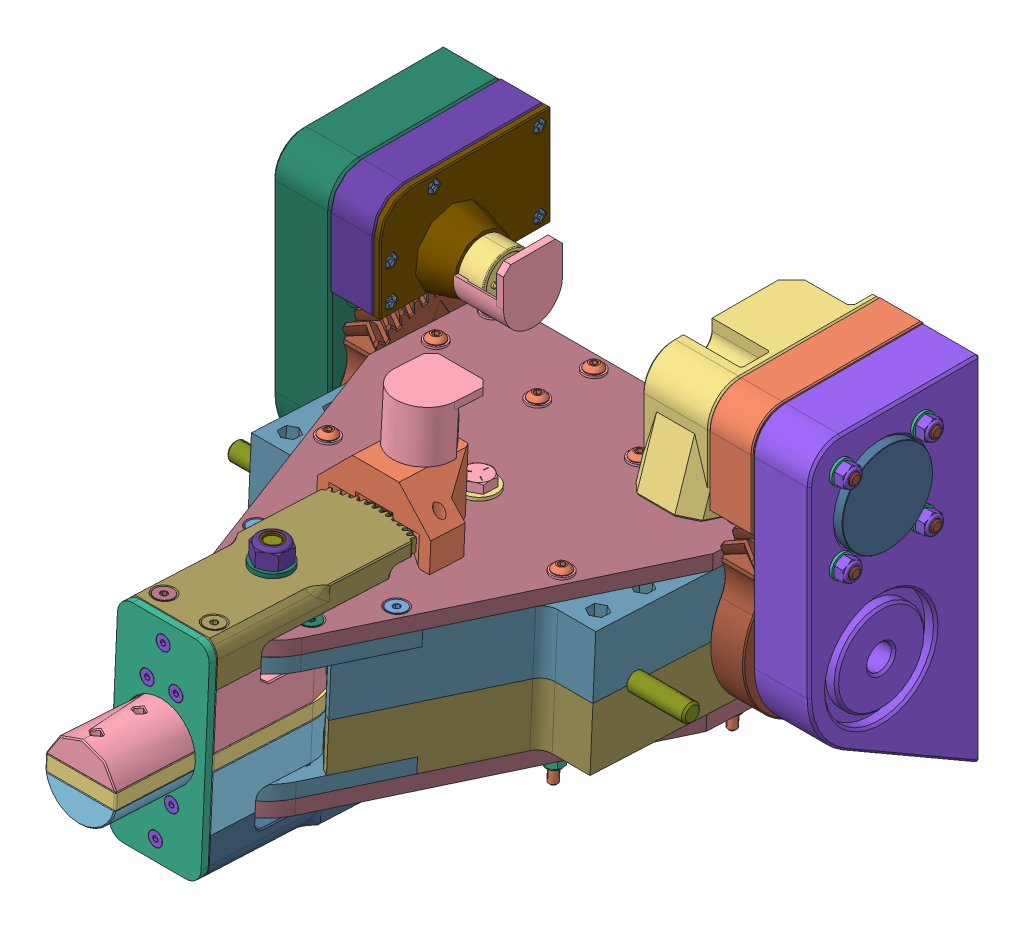
SolidWorks assembly Stick Gimbal Assembly, configuration Default. Lengths in mm.
Overall size (251.4 156.22 281.9).
400 component instances, 76 part files, 23 mates.
Components (placement in the parent):
- Stick Roll Axis Box Assembly-1: Stick Roll Axis Box Assembly [Default] at (0 0 43.8404) x (1 0 0) z (0 0.047106 0.99889) size (220 126.88 270.74)
  - Scissor Arm A Asmbly-1: Scissor Arm A Asmbly [Default] at origin size (38.52 47.7 135.26)
    - Scissor Arm A Link-1: Scissor Arm A Link [Default] at origin size (38.52 3.17 135.26)
    - Scissor Arm A Block-1: Scissor Arm A Block [Default] at origin size (16.74 30.53 64.54)
    - Scissor Arm A Link-2: Scissor Arm A Link [Default] at (0 33.7 0) size (38.52 3.17 135.26)
    - Scissor Cushion-1: Scissor Cushion [Default] at origin size (3.55 36.88 24.93)
    - 93475A230-1: 93475A230 [Default] at (12.7 -18.4375 108.6134) x (1 0 0) z (0 -1 0) size (9 9 0.9)
    - 93475A230-2: 93475A230 [Default] at (17.34 -18.4375 56.0398) x (1 0 0) z (0 -1 0) size (9 9 0.9)
    - 93475A230-3: 93475A230 [Default] at (17.34 -19.3375 56.0398) x (1 0 0) z (0 -1 0) size (9 9 0.9)
    - 93475A230-4: 93475A230 [Default] at (12.7 -19.3375 108.6134) x (1 0 0) z (0 -1 0) size (9 9 0.9)
    - 92095A205-1: 92095A205 [Default] at (12.7 -22.4375 108.6134) x (1 0 0) z (0 -1 0) size (7.65 7.69 47.7)
    - 92095A205-2: 92095A205 [Default] at (17.34 -22.4375 56.0398) x (1 0 0) z (0 -1 0) size (7.65 7.69 47.7)
    - 93475A230-5: 93475A230 [Default] at (12.7 18.4375 108.6134) x (1 0 0) z (0 1 0) size (9 9 0.9)
    - 93475A230-6: 93475A230 [Default] at (17.34 18.4375 56.0398) x (1 0 0) z (0 1 0) size (9 9 0.9)
    - 93625A150-1: 93625A150 [Default] at (12.7 19.3375 108.6134) x (1 0 0) z (0 1 0) size (7 8.08 5)
      - 93625A150_2-1: 93625A150_2 [Default] at origin size (7 8.08 5)
      - 93625A150-1: 93625A150 [Default] at origin size (6.53 6.53 0.53)
    - 93625A150-2: 93625A150 [Default] at (17.34 19.3375 56.0398) x (1 0 0) z (0 1 0) size (7 8.08 5)
      - 93625A150_2-1: 93625A150_2 [Default] at origin size (7 8.08 5)
      - 93625A150-1: 93625A150 [Default] at origin size (6.53 6.53 0.53)
  - Scissor Arm B Asmbly-1: Scissor Arm B Asmbly [Default] at origin size (38.52 47.7 135.26)
    - Scissor Arm B Link Upper-1: Scissor Arm B Link Upper [Default] at origin size (37.06 3.18 116.32)
    - Scissor Arm B Link Spacer-1: Scissor Arm B Link Spacer [Default] at origin size (16.74 2.2 64.54)
    - Scissor Arm B Link Lower-1: Scissor Arm B Link Lower [Default] at origin size (18.2 3.18 83.47)
    - Scissor Arm B Block-1: Scissor Arm B Block [Default] at origin size (16.74 19.78 64.54)
    - Scissor Arm B Link Lower-2: Scissor Arm B Link Lower [Default] at (0 33.7 0) size (18.2 3.18 83.47)
    - Scissor Arm B Link Spacer-2: Scissor Arm B Link Spacer [Default] at (0 28.325 0) size (16.74 2.2 64.54)
    - Scissor Arm B Link Upper-2: Scissor Arm B Link Upper [Default] at (0 22.95 0) size (37.06 3.18 116.32)
    - Scissor Cushion-1: Scissor Cushion [Default] x (-1 0 0) z (0 0 1) size (3.55 36.88 24.93)
    - 93475A230-1: 93475A230 [Default] at (-12.7 -18.4375 108.6134) x (1 0 0) z (0 -1 0) size (9 9 0.9)
    - 93475A230-2: 93475A230 [Default] at (-17.34 -18.4375 56.0398) x (1 0 0) z (0 -1 0) size (9 9 0.9)
    - 93475A230-3: 93475A230 [Default] at (-12.7 -19.3375 108.6134) x (1 0 0) z (0 -1 0) size (9 9 0.9)
    - 93475A230-4: 93475A230 [Default] at (-17.34 -19.3375 56.0398) x (1 0 0) z (0 -1 0) size (9 9 0.9)
    - 92095A205-1: 92095A205 [Default] at (-12.7 -22.4375 108.6134) x (1 0 0) z (0 -1 0) size (7.65 7.69 47.7)
    - 92095A205-2: 92095A205 [Default] at (-17.34 -22.4375 56.0398) x (1 0 0) z (0 -1 0) size (7.65 7.69 47.7)
    - 93475A230-5: 93475A230 [Default] at (-17.34 18.4375 56.0398) x (1 0 0) z (0 1 0) size (9 9 0.9)
    - 93475A230-6: 93475A230 [Default] at (-12.7 18.4375 108.6134) x (1 0 0) z (0 1 0) size (9 9 0.9)
    - 93625A150-1: 93625A150 [Default] at (-17.34 19.3375 56.0398) x (1 0 0) z (0 1 0) size (7 8.08 5)
      - 93625A150_2-1: 93625A150_2 [Default] at origin size (7 8.08 5)
      - 93625A150-1: 93625A150 [Default] at origin size (6.53 6.53 0.53)
    - 93625A150-2: 93625A150 [Default] at (-12.7 19.3375 108.6134) x (1 0 0) z (0 1 0) size (7 8.08 5)
      - 93625A150_2-1: 93625A150_2 [Default] at origin size (7 8.08 5)
      - 93625A150-1: 93625A150 [Default] at origin size (6.53 6.53 0.53)
  - Main Casing Asmbly-1: Main Casing Asmbly [Default] at origin size (220 70.89 189.11)
    - Main Casing A Pre-Asmbly-1: Main Casing A Pre-Asmbly [Default] at (0 141.5449 -37.4581) x (1 0 0) z (0 -0.045363 0.998971) size (152.4 35.57 187.69)
      - Main Casing A-1: Main Casing A [Default] at (0 -139.7 43.8404) x (1 0 0) z (0 0.045363 0.998971) size (152.4 27.13 186.65)
      - 93625A150-1: 93625A150 [Default] at (30.8014 -142.8781 172.2532) x (0.927184 0.016993 0.374221) z (0 0.998971 -0.045363) size (7 8.08 5)
        - 93625A150_2-1: 93625A150_2 [Default] at origin size (7 8.08 5)
        - 93625A150-1: 93625A150 [Default] at origin size (6.53 6.53 0.53)
      - 93625A150-2: 93625A150 [Default] at (-30.8014 -142.8781 172.2532) x (0.927184 -0.016993 -0.374221) z (0 0.998971 -0.045363) size (7 8.08 5)
        - 93625A150_2-1: 93625A150_2 [Default] at origin size (7 8.08 5)
        - 93625A150-1: 93625A150 [Default] at origin size (6.53 6.53 0.53)
      - 94180A351-1: 94180A351 [Default] at (76.2 -154.6945 63.5909) x (0 0.045363 0.998971) z (1 0 0) size (6.35 6.35 4.7)
      - 94180A351-2: 94180A351 [Default] at (76.2 -156.4228 25.5301) x (0 0.045363 0.998971) z (1 0 0) size (6.35 6.35 4.7)
      - 94180A351-3: 94180A351 [Default] at (-76.2 -154.6945 63.5909) x (0 -0.045363 -0.998971) z (-1 0 0) size (6.35 6.35 4.7)
      - 94180A351-4: 94180A351 [Default] at (-76.2 -156.4228 25.5301) x (0 -0.045363 -0.998971) z (-1 0 0) size (6.35 6.35 4.7)
    - Main Casing B Pre-Asmbly-1: Main Casing B Pre-Asmbly [Default] at (0 141.5449 -37.4581) x (1 0 0) z (0 -0.045363 0.998971) size (152.4 35.57 187.69)
      - Main Casing B-1: Main Casing B [Default] at (0 -139.7 43.8404) x (1 0 0) z (0 0.045363 0.998971) size (152.4 27.13 186.65)
      - 93625A150-1: 93625A150 [Default] at (-30.8014 -124.8966 171.4366) x (0.927184 -0.016993 -0.374221) z (0 -0.998971 0.045363) size (7 8.08 5)
        - 93625A150_2-1: 93625A150_2 [Default] at origin size (7 8.08 5)
        - 93625A150-1: 93625A150 [Default] at origin size (6.53 6.53 0.53)
      - 93625A150-2: 93625A150 [Default] at (30.8014 -124.8966 171.4366) x (0.927184 0.016993 0.374221) z (0 -0.998971 0.045363) size (7 8.08 5)
        - 93625A150_2-1: 93625A150_2 [Default] at origin size (7 8.08 5)
        - 93625A150-1: 93625A150 [Default] at origin size (6.53 6.53 0.53)
      - 93625A150-3: 93625A150 [Default] at (26.018 -120.7292 183.0242) x (0.927184 0.016993 0.374221) z (0 0.998971 -0.045363) size (7 8.08 5)
        - 93625A150_2-1: 93625A150_2 [Default] at origin size (7 8.08 5)
        - 93625A150-1: 93625A150 [Default] at origin size (6.53 6.53 0.53)
      - 93625A150-4: 93625A150 [Default] at (-26.018 -120.7292 183.0242) x (0.927184 -0.016993 -0.374221) z (0 0.998971 -0.045363) size (7 8.08 5)
        - 93625A150_2-1: 93625A150_2 [Default] at origin size (7 8.08 5)
        - 93625A150-1: 93625A150 [Default] at origin size (6.53 6.53 0.53)
      - 93625A150-5: 93625A150 [Default] at (-68.2 -128.2463 119.4387) x (1 0 0) z (0 0.998971 -0.045363) size (7 8.08 5)
        - 93625A150_2-1: 93625A150_2 [Default] at origin size (7 8.08 5)
        - 93625A150-1: 93625A150 [Default] at origin size (6.53 6.53 0.53)
      - 93625A150-6: 93625A150 [Default] at (-68.2 -129.1536 99.4592) x (1 0 0) z (0 0.998971 -0.045363) size (7 8.08 5)
        - 93625A150_2-1: 93625A150_2 [Default] at origin size (7 8.08 5)
        - 93625A150-1: 93625A150 [Default] at origin size (6.53 6.53 0.53)
      - 93625A150-7: 93625A150 [Default] at (68.2 -128.2463 119.4387) x (1 0 0) z (0 0.998971 -0.045363) size (7 8.08 5)
        - 93625A150_2-1: 93625A150_2 [Default] at origin size (7 8.08 5)
        - 93625A150-1: 93625A150 [Default] at origin size (6.53 6.53 0.53)
      - 93625A150-8: 93625A150 [Default] at (68.2 -129.1536 99.4592) x (1 0 0) z (0 0.998971 -0.045363) size (7 8.08 5)
        - 93625A150_2-1: 93625A150_2 [Default] at origin size (7 8.08 5)
        - 93625A150-1: 93625A150 [Default] at origin size (6.53 6.53 0.53)
      - 94180A351-1: 94180A351 [Default] at (-76.2 -122.9772 62.1507) x (0 -0.045363 -0.998971) z (-1 0 0) size (6.35 6.35 4.7)
      - 94180A351-2: 94180A351 [Default] at (-76.2 -124.7055 24.0899) x (0 -0.045363 -0.998971) z (-1 0 0) size (6.35 6.35 4.7)
      - 94180A351-3: 94180A351 [Default] at (76.2 -122.9772 62.1507) x (0 0.045363 0.998971) z (1 0 0) size (6.35 6.35 4.7)
      - 94180A351-4: 94180A351 [Default] at (76.2 -124.7055 24.0899) x (0 0.045363 0.998971) z (1 0 0) size (6.35 6.35 4.7)
    - Pitch Axis Rod-1: Pitch Axis Rod [Default] at origin size (220 10 10)
    - 91310A544-1: 91310A544 [Default] at (56.2 0 66.04) x (0 0 1) z (-1 0 0) size (13 15.01 50.3)
    - 91310A544-2: 91310A544 [Default] at (-56.2 0 66.04) x (0 0 -1) z (1 0 0) size (13 15.01 50.3)
    - 57485K68-1: 57485K68 [Default] at (49.45 0 0) x (0 1 0) z (-1 0 0) size (22 22 10)
      - 57485K68-1: 57485K68 [Default] at origin size (22 22 10)
      - 57485K68_2-1: 57485K68_2 [Default] at origin size (4.9 5 4.9)
    - 57485K68-2: 57485K68 [Default] at (-39.45 0 0) x (0 1 0) z (-1 0 0) size (22 22 10)
      - 57485K68-1: 57485K68 [Default] at origin size (22 22 10)
      - 57485K68_2-1: 57485K68_2 [Default] at origin size (4.9 5 4.9)
    - 57485K68-3: 57485K68 [Default] at (5 0 0) x (0 1 0) z (-1 0 0) size (22 22 10)
      - 57485K68-1: 57485K68 [Default] at origin size (22 22 10)
      - 57485K68_2-1: 57485K68_2 [Default] at origin size (4.9 5 4.9)
    - 91390A121-1: 91390A121 [Default] at (44.45 0 -9.9396) x (1 0 0) z (0 0 -1) size (4.9 4.9 10.14)
    - 91390A121-2: 91390A121 [Default] at (-44.45 0 -9.9396) x (1 0 0) z (0 0 -1) size (4.9 4.9 10.14)
    - 91390A121-3: 91390A121 [Default] at (0 0 -9.9396) x (1 0 0) z (0 0 -1) size (4.9 4.9 10.14)
    - 92125A205-1: 92125A205 [Default] at (-68.2 -26.9875 76.04) x (1 0 0) z (0 -1 0) size (8 8 40.14)
    - 92125A205-2: 92125A205 [Default] at (-68.2 -26.9875 56.04) x (1 0 0) z (0 -1 0) size (8 8 40.14)
    - 92125A205-3: 92125A205 [Default] at (68.2 -26.9875 76.04) x (1 0 0) z (0 -1 0) size (8 8 40.14)
    - 92125A205-4: 92125A205 [Default] at (68.2 -26.9875 56.04) x (1 0 0) z (0 -1 0) size (8 8 40.14)
    - 92125A205-5: 92125A205 [Default] at (-26.018 -20.6375 139.9011) x (1 0 0) z (0 -1 0) size (8 8 40.14)
    - 92125A205-6: 92125A205 [Default] at (26.018 -20.6375 139.9011) x (1 0 0) z (0 -1 0) size (8 8 40.14)
  - Pivoting Assembly-1: Pivoting Assembly [Default] at origin size (42.82 89.97 158.75)
    - Pivot Mid Plate-1: Pivot Mid Plate [Default] at origin size (40.64 6.35 158.75)
    - Pivot Block A-1: Pivot Block A [Default] at origin size (41.73 24.41 158.75)
    - Pivot Block B-1: Pivot Block B [Default] at origin size (41.73 24.41 158.75)
    - Pivot Top Plate-1: Pivot Top Plate [Default] at origin size (40.64 89.97 3.17)
    - 94180A331-1: 94180A331 [Default] at (-6.35 -20.8575 197.7644) size (5.56 5.56 3.8)
    - 94180A331-2: 94180A331 [Default] at (6.35 -20.8575 197.7644) size (5.56 5.56 3.8)
    - 94180A331-3: 94180A331 [Default] at (-6.35 20.8575 197.7644) size (5.56 5.56 3.8)
    - 94180A331-4: 94180A331 [Default] at (6.35 20.8575 197.7644) size (5.56 5.56 3.8)
    - 91294A130-1: 91294A130 [Default] at (-6.35 -20.8575 200.9394) size (6 6 10.12)
    - 91294A130-2: 91294A130 [Default] at (6.35 -20.8575 200.9394) size (6 6 10.12)
    - 91294A130-3: 91294A130 [Default] at (-6.35 20.8575 200.9394) size (6 6 10.12)
    - 91294A130-4: 91294A130 [Default] at (6.35 20.8575 200.9394) size (6 6 10.12)
    - 94180A351-1: 94180A351 [Default] at (-11.1125 -27.2075 189.8269) x (1 0 0) z (0 -1 0) size (6.35 6.35 4.7)
    - 94180A351-2: 94180A351 [Default] at (11.1125 27.2075 189.8269) x (1 0 0) z (0 1 0) size (6.35 6.35 4.7)
    - 93625A150-1: 93625A150 [Default] at (-11.1125 -3.175 189.8269) x (1 0 0) z (0 -1 0) size (7 8.08 5)
      - 93625A150_2-1: 93625A150_2 [Default] at origin size (7 8.08 5)
      - 93625A150-1: 93625A150 [Default] at origin size (6.53 6.53 0.53)
    - 93625A150-2: 93625A150 [Default] at (11.1125 3.175 189.8269) x (1 0 0) z (0 1 0) size (7 8.08 5)
      - 93625A150_2-1: 93625A150_2 [Default] at origin size (7 8.08 5)
      - 93625A150-1: 93625A150 [Default] at origin size (6.53 6.53 0.53)
    - 93625A150-3: 93625A150 [Default] at (-11.1125 -9.8438 170.7769) x (1 0 0) z (0 -1 0) size (7 8.08 5)
      - 93625A150_2-1: 93625A150_2 [Default] at origin size (7 8.08 5)
      - 93625A150-1: 93625A150 [Default] at origin size (6.53 6.53 0.53)
    - 93625A150-4: 93625A150 [Default] at (11.1125 -9.8438 170.7769) x (1 0 0) z (0 -1 0) size (7 8.08 5)
      - 93625A150_2-1: 93625A150_2 [Default] at origin size (7 8.08 5)
      - 93625A150-1: 93625A150 [Default] at origin size (6.53 6.53 0.53)
    - 92125A204-1: 92125A204 [Default] at (11.1125 19.8438 170.7769) x (1 0 0) z (0 1 0) size (8 8 35.14)
    - 92125A204-2: 92125A204 [Default] at (-11.1125 19.8438 170.7769) x (1 0 0) z (0 1 0) size (8 8 35.14)
  - Roll Damper Arm A Asmbly-1: Roll Damper Arm A Asmbly [Default] at (0 141.5449 -37.4581) x (1 0 0) z (0 -0.045363 0.998971) size (44.3 24.94 94.29)
    - Roll Damper Arm A-1: Roll Damper Arm A [Default] at (0 -177.6864 199.0377) x (-1 0 0) z (0 0.998971 -0.045363) size (44.3 93.45 20.73)
    - 94180A502-1: 94180A502 [Default] at (0 -167.4235 243.0675) x (-1 0 0) z (0 0.045363 0.998971) size (5.56 5.56 3.81)
  - Roll Damper Arm B Asmbly-1: Roll Damper Arm B Asmbly [Default] at (0 44.9875 153.3144) x (1 0 0) z (0 -1 0) size (44.3 93.45 20.73)
    - Roll Damper Arm B-1: Roll Damper Arm B [Default] at origin size (44.3 93.45 20.73)
    - 94180A502-1: 94180A502 [Default] at (0 44.45 8.255) x (1 0 0) z (0 1 0) size (5.56 5.56 3.81)
  - Fwd Plate Assembly-1: Fwd Plate Assembly [Default] at origin size (152.4 23.35 210.99)
    - Main Plate Sub Asmbly-1: Main Plate Sub Asmbly [Default] at origin size (152.4 12.84 210.99)
      - Main Plate-1: Main Plate [Default] at origin size (152.4 6.35 210.99)
      - Bearing Plate-1: Bearing Plate [Default] at origin size (78.15 6.35 60.33)
      - 91294A192 - M4 x 0.7 mm, 12 mm Long Hex Drive Flat Head Screw-1: 91294A192 - M4 x 0.7 mm, 12 mm Long Hex Drive Flat Head Screw [Default] at (0 -33.3375 171.3144) x (1 0 0) z (0 -1 0) size (8 8 12.14)
      - 91294A192 - M4 x 0.7 mm, 12 mm Long Hex Drive Flat Head Screw-2: 91294A192 - M4 x 0.7 mm, 12 mm Long Hex Drive Flat Head Screw [Default] at (-18 -33.3375 153.3144) x (1 0 0) z (0 -1 0) size (8 8 12.14)
      - 91294A192 - M4 x 0.7 mm, 12 mm Long Hex Drive Flat Head Screw-3: 91294A192 - M4 x 0.7 mm, 12 mm Long Hex Drive Flat Head Screw [Default] at (18 -33.3375 153.3144) x (1 0 0) z (0 -1 0) size (8 8 12.14)
      - 8x22x7+Bearing+-+6082Z-8x22x7_6082Z-8x22x7-1: 8x22x7+Bearing+-+6082Z-8x22x7_6082Z-8x22x7 [Default] at (0 -29.8375 153.3144) x (1 0 0) z (0 -1 0) size (22 22 7.01)
    - FRT-D2-152-G1-1: FRT-D2-152-G1 [Default] at (0 -24.9875 99.3144) x (1 0 0) z (0 -1 0) size (50 25 19)
      - FRT-D2-152-1: FRT-D2-152 [Default] at origin size (50 25 19)
      - FRT-D2-G1 12mm Gear-1: FRT-D2-G1 12mm Gear [Default] at (0 0 14) x (0 -1 0) z (0 0 1) size (14 14 5)
    - 93475A230-1: 93475A230 [Default] at (-20 -33.3375 99.3144) x (1 0 0) z (0 -1 0) size (9 9 0.9)
    - 93475A230-2: 93475A230 [Default] at (20 -33.3375 99.3144) x (1 0 0) z (0 -1 0) size (9 9 0.9)
    - 93625A150-1: 93625A150 [Default] at (-20 -34.2375 99.3144) x (1 0 0) z (0 -1 0) size (7 8.08 5)
      - 93625A150_2-1: 93625A150_2 [Default] at origin size (7 8.08 5)
      - 93625A150-1: 93625A150 [Default] at origin size (6.53 6.53 0.53)
    - 93625A150-2: 93625A150 [Default] at (20 -34.2375 99.3144) x (1 0 0) z (0 -1 0) size (7 8.08 5)
      - 93625A150_2-1: 93625A150_2 [Default] at origin size (7 8.08 5)
      - 93625A150-1: 93625A150 [Default] at origin size (6.53 6.53 0.53)
    - 91239A150-1: 91239A150 [Default] at (20 -22.7875 99.3144) x (1 0 0) z (0 1 0) size (7.65 7.69 18.7)
    - 91239A150-2: 91239A150 [Default] at (-20 -22.7875 99.3144) x (1 0 0) z (0 1 0) size (7.65 7.69 18.7)
  - Aft Plate Assembly-1: Aft Plate Assembly [Default] x (-1 0 0) z (0 0 1) size (152.4 54.07 210.99)
    - Main Plate Sub Asmbly_1-1: Main Plate Sub Asmbly_1 [Default] at origin size (152.4 12.84 210.99)
      - Main Plate-1: Main Plate [Default] at origin size (152.4 6.35 210.99)
      - Bearing Plate-1: Bearing Plate [Default] at origin size (78.15 6.35 60.33)
      - 91294A192 - M4 x 0.7 mm, 12 mm Long Hex Drive Flat Head Screw-1: 91294A192 - M4 x 0.7 mm, 12 mm Long Hex Drive Flat Head Screw [Default] at (0 -33.3375 171.3144) x (1 0 0) z (0 -1 0) size (8 8 12.14)
      - 91294A192 - M4 x 0.7 mm, 12 mm Long Hex Drive Flat Head Screw-2: 91294A192 - M4 x 0.7 mm, 12 mm Long Hex Drive Flat Head Screw [Default] at (-18 -33.3375 153.3144) x (1 0 0) z (0 -1 0) size (8 8 12.14)
      - 91294A192 - M4 x 0.7 mm, 12 mm Long Hex Drive Flat Head Screw-3: 91294A192 - M4 x 0.7 mm, 12 mm Long Hex Drive Flat Head Screw [Default] at (18 -33.3375 153.3144) x (1 0 0) z (0 -1 0) size (8 8 12.14)
      - 8x22x7+Bearing+-+6082Z-8x22x7_6082Z-8x22x7-1: 8x22x7+Bearing+-+6082Z-8x22x7_6082Z-8x22x7 [Default] at (0 -29.8375 153.3144) x (1 0 0) z (0 -1 0) size (22 22 7.01)
    - FRT-D2-152-G1_1-1: FRT-D2-152-G1_1 [Default] at (0 -24.9875 99.3144) x (-1 0 0) z (0 -1 0) size (50 25 19)
      - FRT-D2-152-1: FRT-D2-152 [Default] at origin size (50 25 19)
      - FRT-D2-G1 12mm Gear-2: FRT-D2-G1 12mm Gear [Default] at (0 0 14) x (0 -1 0) z (0 0 1) size (14 14 5)
    - 91239A150-1: 91239A150 [Default] at (20 -22.7875 99.3144) x (-1 0 0) z (0 1 0) size (7.65 7.69 18.7)
    - 91239A150-2: 91239A150 [Default] at (-20 -22.7875 99.3144) x (-1 0 0) z (0 1 0) size (7.65 7.69 18.7)
    - Roll Sensor Asmbly-1: Roll Sensor Asmbly [Default] x (-1 0 0) z (0 0 1) size (50.16 41.37 31.85)
      - Roll Sensor Mount Main-1: Roll Sensor Mount Main [Default] at origin size (50.16 27.53 31.75)
      - 94180A351-1: 94180A351 [Default] at (-20 33.3375 99.3144) x (1 0 0) z (0 -1 0) size (6.35 6.35 4.7)
      - 94180A351-2: 94180A351 [Default] at (20 33.3375 99.3144) x (1 0 0) z (0 -1 0) size (6.35 6.35 4.7)
      - 6127V1AxxxL.5FS-1: 6127V1AxxxL.5FS [6127V1A360L.5FS] at (0 61.2423 87.3281) x (1 0 0) z (0 0.011977 0.999928) size (22.23 35.66 22.23)
      - Roll Damper Gear-1: Roll Damper Gear [Default] at (0 38.9173 87.5956) x (-1 0 0) z (0 0.999928 -0.011977) size (14 14 10)
  - Scissor Stop-1: Scissor Stop [Default] at origin size (20.44 53.98 22.23)
  - 93475A240-1: 93475A240 [Default] at (-19.471 -18.4375 37.1094) x (1 0 0) z (0 -1 0) size (10 10 1.1)
  - 93475A240-2: 93475A240 [Default] at (19.471 -18.4375 37.1094) x (1 0 0) z (0 -1 0) size (10 10 1.1)
  - 93475A240-3: 93475A240 [Default] at (-19.471 19.5375 37.1094) x (1 0 0) z (0 -1 0) size (10 10 1.1)
  - 93475A240-4: 93475A240 [Default] at (19.471 18.4375 37.1094) x (1 0 0) z (0 1 0) size (10 10 1.1)
  - 91239A244-1: 91239A244 [Default] at (-19.471 -22.2875 37.1094) x (1 0 0) z (0 -1 0) size (9.57 9.61 48.38)
  - 91239A244-2: 91239A244 [Default] at (19.471 -22.2875 37.1094) x (1 0 0) z (0 -1 0) size (9.57 9.61 48.38)
  - 93625A200 - M5 x 0.8 mm Nylon-Insert Locknut-1: 93625A200 - M5 x 0.8 mm Nylon-Insert Locknut [Default] at (19.471 19.5375 37.1094) x (1 0 0) z (0 1 0) size (8 9.24 5)
    - 93625A200 - M5 x 0.8 mm Nylon-Insert Locknut_2-1: 93625A200 - M5 x 0.8 mm Nylon-Insert Locknut_2 [Default] at origin size (8 9.24 5)
    - 93625A200 - M5 x 0.8 mm Nylon-Insert Locknut-1: 93625A200 - M5 x 0.8 mm Nylon-Insert Locknut [Default] at origin size (7.53 7.53 0.53)
  - 93625A200 - M5 x 0.8 mm Nylon-Insert Locknut-2: 93625A200 - M5 x 0.8 mm Nylon-Insert Locknut [Default] at (-19.471 19.5375 37.1094) x (1 0 0) z (0 1 0) size (8 9.24 5)
    - 93625A200 - M5 x 0.8 mm Nylon-Insert Locknut_2-1: 93625A200 - M5 x 0.8 mm Nylon-Insert Locknut_2 [Default] at origin size (8 9.24 5)
    - 93625A200 - M5 x 0.8 mm Nylon-Insert Locknut-1: 93625A200 - M5 x 0.8 mm Nylon-Insert Locknut [Default] at origin size (7.53 7.53 0.53)
  - 9654K421 - 1.75 Long, 0.5_ OD, 0.055_ WD Steel Extension Spring with_ Loop Ends-1: 9654K421 - 1.75 Long, 0.5_ OD, 0.055_ WD Steel Extension Spring with_ Loop Ends [Default] at (-1.096 0.0125 37.1094) x (1 0 0) z (0 -1 0) size (44.45 14.38 14.38)
  - 9654K421 - 1.75 Long, 0.5_ OD, 0.055_ WD Steel Extension Spring with_ Loop Ends-2: 9654K421 - 1.75 Long, 0.5_ OD, 0.055_ WD Steel Extension Spring with_ Loop Ends [Default] at (-1.096 -13.9375 37.1094) x (1 0 0) z (0 -1 0) size (44.45 14.38 14.38)
  - 9654K421 - 1.75 Long, 0.5_ OD, 0.055_ WD Steel Extension Spring with_ Loop Ends-3: 9654K421 - 1.75 Long, 0.5_ OD, 0.055_ WD Steel Extension Spring with_ Loop Ends [Default] at (-1.096 13.9625 37.1094) x (1 0 0) z (0 -1 0) size (44.45 14.38 14.38)
  - Pitch Damper Gear Large-1: Pitch Damper Gear Large [Default] at (-83.7 0 0) x (0 0.99889 0.047106) z (1 0 0) size (80.38 66.68 15)
  - Pitch Damper Gear Large-2: Pitch Damper Gear Large [Default] at (83.7 0 0) x (0 0.99889 0.047106) z (1 0 0) size (80.38 66.68 15)
  - 91294A198-1: 91294A198 [Default] at (91.2 -15.9082 19.0223) x (0 -0.047106 0.99889) z (1 0 0) size (8 8 25.14)
  - 91294A198-2: 91294A198 [Default] at (91.2 15.9082 -19.0223) x (0 -0.047106 0.99889) z (1 0 0) size (8 8 25.14)
  - 91294A198-3: 91294A198 [Default] at (91.2 -15.8417 -19.0777) x (0 -0.047106 0.99889) z (1 0 0) size (8 8 25.14)
  - 91294A198-4: 91294A198 [Default] at (91.2 15.8417 19.0777) x (0 0.047106 -0.99889) z (1 0 0) size (8 8 25.14)
  - 91294A198-5: 91294A198 [Default] at (-91.2 15.8417 19.0777) x (0 0.047106 -0.99889) z (-1 0 0) size (8 8 25.14)
  - 91294A198-6: 91294A198 [Default] at (-91.2 -15.8417 -19.0777) x (0 0.047106 -0.99889) z (-1 0 0) size (8 8 25.14)
  - 91294A198-7: 91294A198 [Default] at (-91.2 15.9082 -19.0223) x (0 0.047106 -0.99889) z (-1 0 0) size (8 8 25.14)
  - 91294A198-8: 91294A198 [Default] at (-91.2 -15.9082 19.0223) x (0 0.047106 -0.99889) z (-1 0 0) size (8 8 25.14)
  - 92125A373-1: 92125A373 [Default] at (-11.1125 44.9875 189.8269) x (1 0 0) z (0 1 0) size (8 8 55.09)
  - 92125A373-2: 92125A373 [Default] at (11.1125 -44.9875 189.8269) x (1 0 0) z (0 -1 0) size (8 8 55.09)
  - 91294A198-9: 91294A198 [Default] at (-11.1125 -44.9875 189.8269) x (1 0 0) z (0 -1 0) size (8 8 25.14)
  - 91294A198-10: 91294A198 [Default] at (11.1125 44.9875 189.8269) x (1 0 0) z (0 1 0) size (8 8 25.14)
  - 95630A670-1: 95630A670 [Default] at (0 -7.6875 153.3144) x (1 0 0) z (0 -1 0) size (18 18 2.2)
  - 95630A670-2: 95630A670 [Default] at (0 -13.0625 153.3144) x (1 0 0) z (0 -1 0) size (18 18 2.2)
  - 95630A670-3: 95630A670 [Default] at (0 7.6875 153.3144) x (1 0 0) z (0 1 0) size (18 18 2.2)
  - 95630A670-4: 95630A670 [Default] at (0 13.0625 153.3144) x (1 0 0) z (0 1 0) size (18 18 2.2)
  - 93475A270 - M8 Stainless Steel Washer-1: 93475A270 - M8 Stainless Steel Washer [Default] at (0 34.9875 153.3144) x (1 0 0) z (0 -1 0) size (16 16 1.8)
  - 93475A270 - M8 Stainless Steel Washer-2: 93475A270 - M8 Stainless Steel Washer [Default] at (0 -34.9875 153.3144) x (1 0 0) z (0 1 0) size (16 16 1.8)
  - 91280A174-1: 91280A174 [Default] at (0 -40.9875 153.3144) x (1 0 0) z (0 -1 0) size (13 15.01 100.3)
  - 93475A270 - M8 Stainless Steel Washer-3: 93475A270 - M8 Stainless Steel Washer [Default] at (0 46.7875 153.3144) x (1 0 0) z (0 -1 0) size (16 16 1.8)
  - 90576A117 - M8 x 1.25mm Nylon-Insert Lock Nut-1: 90576A117 - M8 x 1.25mm Nylon-Insert Lock Nut [Default] at (0 46.7875 153.3144) x (1 0 0) z (0 1 0) size (13 15.01 8)
    - 90576A117 - M8 x 1.25mm Nylon-Insert Lock Nut_2-1: 90576A117 - M8 x 1.25mm Nylon-Insert Lock Nut_2 [Default] at origin size (13 15.01 8)
    - 90576A117 - M8 x 1.25mm Nylon-Insert Lock Nut-1: 90576A117 - M8 x 1.25mm Nylon-Insert Lock Nut [Default] at origin size (12.54 12.54 1.03)
  - 91294A130-1: 91294A130 [Default] at (0 -36.7325 200.9394) size (6 6 10.12)
  - 91294A130-2: 91294A130 [Default] at (0 36.7325 200.9394) size (6 6 10.12)
  - 92125A203-1: 92125A203 [Default] at (-30.8014 33.3375 128.1364) x (1 0 0) z (0 1 0) size (8 8 30.14)
  - 92125A203-2: 92125A203 [Default] at (-30.8014 -33.3375 128.1364) x (1 0 0) z (0 -1 0) size (8 8 30.14)
  - 92125A203-3: 92125A203 [Default] at (30.8014 -33.3375 128.1364) x (1 0 0) z (0 -1 0) size (8 8 30.14)
  - 92125A203-4: 92125A203 [Default] at (30.8014 33.3375 128.1364) x (1 0 0) z (0 1 0) size (8 8 30.14)
  - 93475A230-1: 93475A230 [Default] at (67.5 33.3375 12.5) x (1 0 0) z (0 1 0) size (9 9 0.9)
  - 93475A230-2: 93475A230 [Default] at (67.5 33.3375 -12.5) x (1 0 0) z (0 1 0) size (9 9 0.9)
  - 93475A230-3: 93475A230 [Default] at (22.5 33.3375 12.5) x (1 0 0) z (0 1 0) size (9 9 0.9)
  - 93475A230-4: 93475A230 [Default] at (22.5 33.3375 -12.5) x (1 0 0) z (0 1 0) size (9 9 0.9)
  - 93475A230-5: 93475A230 [Default] at (-22.5 33.3375 12.5) x (1 0 0) z (0 1 0) size (9 9 0.9)
  - 93475A230-6: 93475A230 [Default] at (-22.5 33.3375 -12.5) x (1 0 0) z (0 1 0) size (9 9 0.9)
  - 93475A230-7: 93475A230 [Default] at (-67.5 33.3375 12.5) x (1 0 0) z (0 1 0) size (9 9 0.9)
  - 93475A230-8: 93475A230 [Default] at (-67.5 33.3375 -12.5) x (1 0 0) z (0 1 0) size (9 9 0.9)
  - 93475A230-9: 93475A230 [Default] at (51.7 33.3375 76.04) x (1 0 0) z (0 1 0) size (9 9 0.9)
  - 93475A230-10: 93475A230 [Default] at (-51.7 33.3375 76.04) x (1 0 0) z (0 1 0) size (9 9 0.9)
  - 93475A230-11: 93475A230 [Default] at (-51.7 -34.2375 76.04) x (1 0 0) z (0 1 0) size (9 9 0.9)
  - 93475A230-12: 93475A230 [Default] at (67.5 -34.2375 -12.5) x (1 0 0) z (0 1 0) size (9 9 0.9)
  - 93475A230-13: 93475A230 [Default] at (51.7 -34.2375 76.04) x (1 0 0) z (0 1 0) size (9 9 0.9)
  - 93475A230-14: 93475A230 [Default] at (67.5 -34.2375 12.5) x (1 0 0) z (0 1 0) size (9 9 0.9)
  - 93475A230-15: 93475A230 [Default] at (-22.5 -34.2375 12.5) x (1 0 0) z (0 1 0) size (9 9 0.9)
  - 93475A230-16: 93475A230 [Default] at (22.5 -34.2375 12.5) x (1 0 0) z (0 1 0) size (9 9 0.9)
  - 93475A230-17: 93475A230 [Default] at (22.5 -34.2375 -12.5) x (1 0 0) z (0 1 0) size (9 9 0.9)
  - 93475A230-18: 93475A230 [Default] at (-22.5 -34.2375 -12.5) x (1 0 0) z (0 1 0) size (9 9 0.9)
  - 93475A230-19: 93475A230 [Default] at (-67.5 -34.2375 -12.5) x (1 0 0) z (0 1 0) size (9 9 0.9)
  - 93475A230-20: 93475A230 [Default] at (-67.5 -34.2375 12.5) x (1 0 0) z (0 1 0) size (9 9 0.9)
  - 92095A173-1: 92095A173 [Default] at (67.5 34.2375 12.5) x (1 0 0) z (0 1 0) size (7.65 7.69 82.7)
  - 92095A173-2: 92095A173 [Default] at (67.5 34.2375 -12.5) x (1 0 0) z (0 1 0) size (7.65 7.69 82.7)
  - 92095A173-3: 92095A173 [Default] at (22.5 34.2375 -12.5) x (1 0 0) z (0 1 0) size (7.65 7.69 82.7)
  - 92095A173-4: 92095A173 [Default] at (22.5 34.2375 12.5) x (1 0 0) z (0 1 0) size (7.65 7.69 82.7)
  - 92095A173-5: 92095A173 [Default] at (-67.5 34.2375 12.5) x (1 0 0) z (0 1 0) size (7.65 7.69 82.7)
  - 92095A173-6: 92095A173 [Default] at (-22.5 34.2375 -12.5) x (1 0 0) z (0 1 0) size (7.65 7.69 82.7)
  - 92095A173-7: 92095A173 [Default] at (-67.5 34.2375 -12.5) x (1 0 0) z (0 1 0) size (7.65 7.69 82.7)
  - 92095A173-8: 92095A173 [Default] at (-22.5 34.2375 12.5) x (1 0 0) z (0 1 0) size (7.65 7.69 82.7)
  - 92095A173-9: 92095A173 [Default] at (51.7 34.2375 76.04) x (1 0 0) z (0 1 0) size (7.65 7.69 82.7)
  - 92095A173-10: 92095A173 [Default] at (-51.7 34.2375 76.04) x (1 0 0) z (0 1 0) size (7.65 7.69 82.7)
  - 93625A150-1: 93625A150 [Default] at (67.5 -34.2375 12.5) x (1 0 0) z (0 -1 0) size (7 8.08 5)
    - 93625A150_2-1: 93625A150_2 [Default] at origin size (7 8.08 5)
    - 93625A150-1: 93625A150 [Default] at origin size (6.53 6.53 0.53)
  - 93625A150-2: 93625A150 [Default] at (67.5 -34.2375 -12.5) x (1 0 0) z (0 -1 0) size (7 8.08 5)
    - 93625A150_2-1: 93625A150_2 [Default] at origin size (7 8.08 5)
    - 93625A150-1: 93625A150 [Default] at origin size (6.53 6.53 0.53)
  - 93625A150-3: 93625A150 [Default] at (22.5 -34.2375 -12.5) x (1 0 0) z (0 -1 0) size (7 8.08 5)
    - 93625A150_2-1: 93625A150_2 [Default] at origin size (7 8.08 5)
    - 93625A150-1: 93625A150 [Default] at origin size (6.53 6.53 0.53)
  - 93625A150-4: 93625A150 [Default] at (22.5 -34.2375 12.5) x (1 0 0) z (0 -1 0) size (7 8.08 5)
    - 93625A150_2-1: 93625A150_2 [Default] at origin size (7 8.08 5)
    - 93625A150-1: 93625A150 [Default] at origin size (6.53 6.53 0.53)
  - 93625A150-5: 93625A150 [Default] at (-67.5 -34.2375 12.5) x (1 0 0) z (0 -1 0) size (7 8.08 5)
    - 93625A150_2-1: 93625A150_2 [Default] at origin size (7 8.08 5)
    - 93625A150-1: 93625A150 [Default] at origin size (6.53 6.53 0.53)
  - 93625A150-6: 93625A150 [Default] at (-67.5 -34.2375 -12.5) x (1 0 0) z (0 -1 0) size (7 8.08 5)
    - 93625A150_2-1: 93625A150_2 [Default] at origin size (7 8.08 5)
    - 93625A150-1: 93625A150 [Default] at origin size (6.53 6.53 0.53)
  - 93625A150-7: 93625A150 [Default] at (-22.5 -34.2375 -12.5) x (1 0 0) z (0 -1 0) size (7 8.08 5)
    - 93625A150_2-1: 93625A150_2 [Default] at origin size (7 8.08 5)
